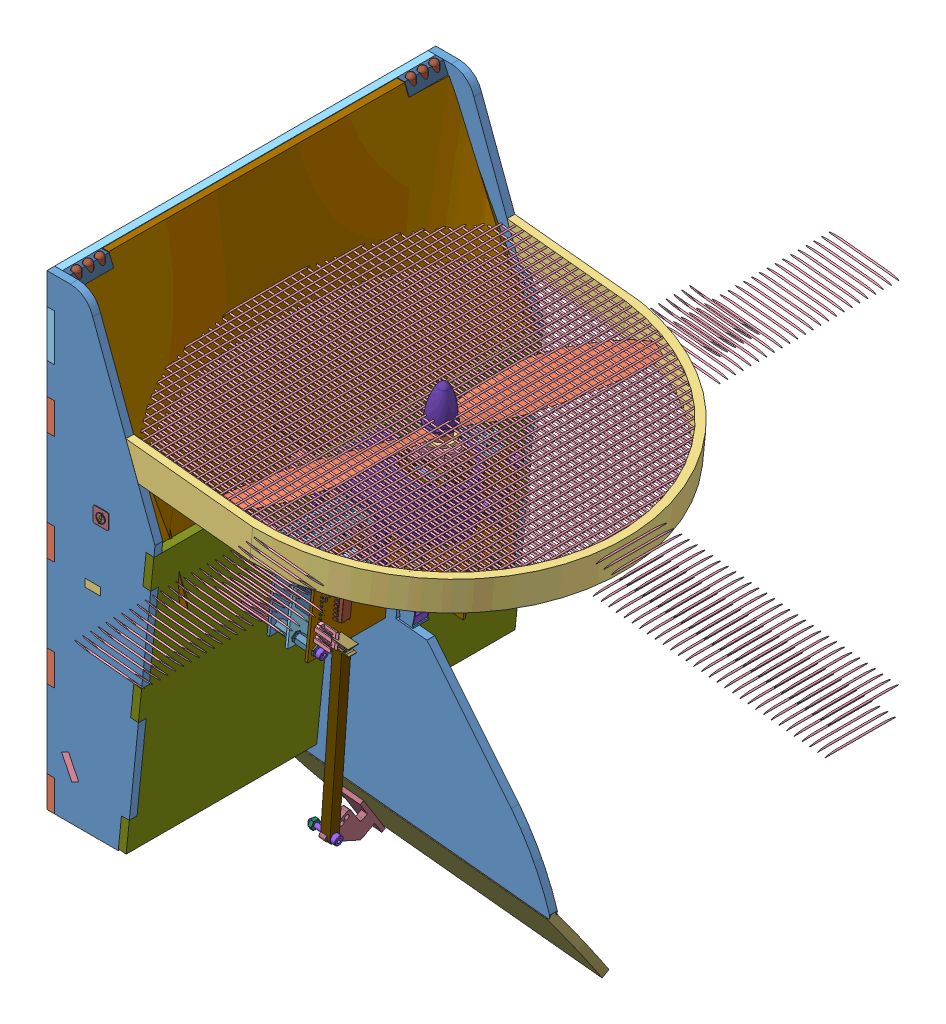
SolidWorks assembly AssTotaleSimu5, configuration Défaut. Lengths in mm.
Overall size (253.25 382.9 251.6).
1779 component instances, 238 part files, 11 mates.
Components (placement in the parent):
- AssStructSimu-1: AssStructSimu [Défaut] at (-125.7658 -1.8483 624.6548) x (1 0 0) z (0 0 -1) size (253.25 324.59 251.6)
  - AssBase-1: AssBase [Défaut] at (36.5482 -71.0398 34.0612) size (86.08 302.3 251.6)
    - AssD-1: AssD [Défaut] at (39.0992 31.0201 8.5) size (69.5 300 22)
      - P1-1: P1 [Défaut] at (-95.5819 194.6656 377.5) size (69.5 300 5)
      - P5-1: P5 [Défaut] at (-100.5819 -35.3344 360.5) x (0 1 0) z (1 0 0) size (230 22 5)
    - AssG-1: AssG [Défaut] at (39.0992 31.0201 -236.5) size (69.5 300 22)
      - P1-1: P1 [Défaut] at (-95.5819 194.6656 377.5) size (69.5 300 5)
      - P5-1: P5 [Défaut] at (-95.5819 -35.3344 399.5) x (0 1 0) z (-1 0 0) size (230 22 5)
    - P7-1: P7 [Défaut] at (-1.4828 89.6857 370.5) x (0 0 -1) z (0 -1 0) size (250 54.5 5)
    - P4-1: P4 [Défaut] at (-63.2363 165.9323 386) x (0 0 -1) z (0.898794 -0.438371 0) size (250 60.5 66.27)
    - P3-1: P3 [Défaut] at (-56.4828 -74.3143 146) x (0 0 1) z (-1 0 0) size (250 70 5)
    - P4b-1: P4b [Défaut] at (-58.7423 163.7404 190) x (0 0 1) z (0.438371 0.898794 0) size (152 56 2)
    - battery-1: battery [Défaut] at (-39.0156 204.1861 197.5) x (0 0 1) z (0.898794 -0.438371 0) size (137 43 30)
    - socket head cap screw 4762_din-1: socket head cap screw 4762_din [EN ISO 4762 M3 x 10 - 10N] at (-27.7008 145.2627 193) x (0.438371 0.898794 0) z (0 0 -1) size (13 5.5 5.5)
    - socket head cap screw 4762_din-2: socket head cap screw 4762_din [EN ISO 4762 M3 x 10 - 10N] at (-27.7008 145.2627 339) x (0.438371 0.898794 0) z (-0.791285 0.385936 -0.474259) size (13 5.5 5.5)
    - socket head cap screw 4762_din-3: socket head cap screw 4762_din [EN ISO 4762 M3 x 10 - 10N] at (-42.0815 152.2766 339) x (0.438371 0.898794 0) z (-0.001489 0.000726 -0.999999) size (13 5.5 5.5)
    - socket head cap screw 4762_din-4: socket head cap screw 4762_din [EN ISO 4762 M3 x 10 - 10N] at (-42.0815 152.2766 193) x (0.438371 0.898794 0) z (-0.031331 0.015281 -0.999392) size (13 5.5 5.5)
    - P11-1: P11 [Défaut] at (-57.5734 -73.9703 146.7843) x (0.005072 0 0.999987) z (0.006197 0.999981 -0.000031) size (240 65 164)
    - AssPhare-1: AssPhare [Défaut] at (-52.8518 -67.6977 411) x (0 1 0) z (0 0 -1) size (35.8 8 25)
      - piece_led-1: piece_led [Défaut] at (-6.6166 -3.631 25) size (7 8 25)
      - LED 5mm-1: LED 5mm [Valor predeterminado] at (-0.1166 0.369 30) x (0 0 1) z (-1 0 0) size (10.06 6 40.8)
      - LED 5mm-2: LED 5mm [Valor predeterminado] at (-0.1166 0.369 37.5) x (0 0 1) z (-1 0 0) size (10.06 6 40.8)
      - LED 5mm-3: LED 5mm [Valor predeterminado] at (-0.1166 0.369 45) x (0 0 1) z (-1 0 0) size (10.06 6 40.8)
    - AssPhare-2: AssPhare [Défaut] at (-52.8518 -67.6977 196) x (0 1 0) z (0 0 -1) size (35.8 8 25)
      - piece_led-1: piece_led [Défaut] at (-6.6166 -3.631 25) size (7 8 25)
      - LED 5mm-1: LED 5mm [Valor predeterminado] at (-0.1166 0.369 30) x (0 0 1) z (-1 0 0) size (10.06 6 40.8)
      - LED 5mm-2: LED 5mm [Valor predeterminado] at (-0.1166 0.369 37.5) x (0 0 1) z (-1 0 0) size (10.06 6 40.8)
      - LED 5mm-3: LED 5mm [Valor predeterminado] at (-0.1166 0.369 45) x (0 0 1) z (-1 0 0) size (10.06 6 40.8)
    - AssLogo-1: AssLogo [Défaut] at (-27.8835 45.1673 148.1054) x (-1 0 0) z (0 0 -1) size (10 10 0.8)
      - logo1-1: logo1 [Défaut] at (-6.5271 -4.4734 6.5054) size (5.8 7.71 0.4)
      - logo2-1: logo2 [Défaut] at (-6.4007 -4.4815 7.1054) size (10 10 0.4)
    - AssLogo-2: AssLogo [Défaut] at (-25.082 45.1673 383.8946) size (10 10 0.8)
      - logo1-1: logo1 [Défaut] at (-6.5271 -4.4734 6.5054) size (5.8 7.71 0.4)
      - logo2-1: logo2 [Défaut] at (-6.4007 -4.4815 7.1054) size (10 10 0.4)
    - support2-1: support2 [Défaut] at (-61.5648 191.7124 276) x (-0.017452 -0.999848 0) z (0.999848 -0.017452 0) size (75 20 10)
    - socket head cap screw 4762_din-5: socket head cap screw 4762_din [EN ISO 4762 M3 x 5 - 5N] at (-61.652 186.7132 269.3333) x (0.999848 -0.017452 0) z (-0.002158 -0.123615 0.992328) size (8 5.5 5.5)
    - socket head cap screw 4762_din-6: socket head cap screw 4762_din [EN ISO 4762 M3 x 5 - 5N] at (-61.652 186.7132 262.6667) x (0.999848 -0.017452 0) z (0 0 1) size (8 5.5 5.5)
    - socket head cap screw 4762_din-7: socket head cap screw 4762_din [EN ISO 4762 M3 x 25 - 18N] at (-55.2963 121.0922 253) x (0 0 1) z (-1 0 0) size (28 5.5 5.5)
    - hex nut style 1 gradeab_din-1: hex nut style 1 gradeab_din [Hexagon Nut ISO 4032 - M3 - W - N] at (-55.2963 121.0922 276) x (-0.923728 -0.383049 0) z (0 0 -1) size (5.5 6.35 2.4)
  - AssToitMot-1: AssToitMot [Défaut] at (-168.5238 43.6961 238.494) x (0 0 -1) z (0.9948 0.101852 0) size (250 207.5 205)
    - AssToit-1: AssToit [Défaut] at (-23.0702 -16.5789 -3.7148) size (250 207.5 205)
      - P8-1: P8 [Défaut] at (-38.4971 122.5921 203.5) size (250 175 5)
      - P12-1: P12 [Défaut] at (-60.4971 -63.4079 265.5) x (1 0 0) z (0 -1 0) size (44.28 76.64 55)
      - P13-1: P13 [Défaut] at (-35.9971 -52.8579 208.5) x (0 0 1) z (-1 0 0) size (64 15.55 5)
      - P10_2-1: P10_2 [Défaut] at (-35.9971 111.5921 171) x (0 0 1) z (-1 0 0) size (188.5 117.6 5)
    - Parallax-Servo_DUMMY-1: Parallax-Servo_DUMMY [Défaut] at (-61.6002 -51.5207 216.6662) x (1 0 0) z (0 1 0) size (20.07 42.67 55.64)
    - socket head cap screw 4762_din-1: socket head cap screw 4762_din [EN ISO 4762 M2.5 x 5 - 5N] at (-51.9272 -76.4868 259.2852) x (0 -1 0) z (-0.546944 0 0.837169) size (7.5 4.5 4.5)
    - socket head cap screw 4762_din-2: socket head cap screw 4762_din [EN ISO 4762 M2.5 x 5 - 5N] at (-61.5672 -76.4868 268.9252) x (0 -1 0) z (-0.546944 0 0.837169) size (7.5 4.5 4.5)
    - socket head cap screw 4762_din-3: socket head cap screw 4762_din [EN ISO 4762 M2.5 x 5 - 5N] at (-71.2072 -76.4868 259.2852) x (0 -1 0) z (-0.546944 0 0.837169) size (7.5 4.5 4.5)
    - socket head cap screw 4762_din-4: socket head cap screw 4762_din [EN ISO 4762 M2.5 x 5 - 5N] at (-61.5672 -76.4868 249.6452) x (0 -1 0) z (-0.546944 0 0.837169) size (7.5 4.5 4.5)
    - AssPhare-1: AssPhare [Défaut] at (8.4328 83.3966 196.1542) x (0 -1 0) z (1 0 0) size (35.8 8 25)
      - piece_led-1: piece_led [Défaut] at (-6.6166 -3.631 25) size (7 8 25)
      - LED 5mm-1: LED 5mm [Valor predeterminado] at (-0.1166 0.369 30) x (0 0 1) z (-1 0 0) size (10.06 6 40.8)
      - LED 5mm-2: LED 5mm [Valor predeterminado] at (-0.1166 0.369 37.5) x (0 0 1) z (-1 0 0) size (10.06 6 40.8)
      - LED 5mm-3: LED 5mm [Valor predeterminado] at (-0.1166 0.369 45) x (0 0 1) z (-1 0 0) size (10.06 6 40.8)
    - AssPhare-2: AssPhare [Défaut] at (-206.5672 83.3966 196.1542) x (0 -1 0) z (1 0 0) size (35.8 8 25)
      - piece_led-1: piece_led [Défaut] at (-6.6166 -3.631 25) size (7 8 25)
      - LED 5mm-1: LED 5mm [Valor predeterminado] at (-0.1166 0.369 30) x (0 0 1) z (-1 0 0) size (10.06 6 40.8)
      - LED 5mm-2: LED 5mm [Valor predeterminado] at (-0.1166 0.369 37.5) x (0 0 1) z (-1 0 0) size (10.06 6 40.8)
      - LED 5mm-3: LED 5mm [Valor predeterminado] at (-0.1166 0.369 45) x (0 0 1) z (-1 0 0) size (10.06 6 40.8)
    - socket head cap screw 4762_din-5: socket head cap screw 4762_din [EN ISO 4762 M3 x 10 - 10N] at (-67.0672 -22.9368 210.2852) x (0 0 -1) z (1 0 0) size (13 5.5 5.5)
    - socket head cap screw 4762_din-6: socket head cap screw 4762_din [EN ISO 4762 M3 x 10 - 10N] at (-56.0672 -72.9868 210.2852) x (0 0 -1) z (1 0 0) size (13 5.5 5.5)
    - socket head cap screw 4762_din-7: socket head cap screw 4762_din [EN ISO 4762 M3 x 10 - 10N] at (-67.0672 -72.9868 210.2852) x (0 0 -1) z (1 0 0) size (13 5.5 5.5)
    - socket head cap screw 4762_din-8: socket head cap screw 4762_din [EN ISO 4762 M3 x 10 - 10N] at (-56.0672 -22.9368 210.2852) x (0 0 -1) z (1 0 0) size (13 5.5 5.5)
    - hex nut style 1 gradeab_din-1: hex nut style 1 gradeab_din [Hexagon Nut ISO 4032 - M3 - W - N] at (-67.0672 -72.9868 197.3852) x (-0.923728 -0.383049 0) z (0 0 -1) size (5.5 6.35 2.4)
    - hex nut style 1 gradeab_din-2: hex nut style 1 gradeab_din [Hexagon Nut ISO 4032 - M3 - W - N] at (-56.0672 -72.9868 199.7852) size (5.5 6.35 2.4)
    - hex nut style 1 gradeab_din-3: hex nut style 1 gradeab_din [Hexagon Nut ISO 4032 - M3 - W - N] at (-67.0672 -22.9368 199.7852) size (5.5 6.35 2.4)
    - hex nut style 1 gradeab_din-4: hex nut style 1 gradeab_din [Hexagon Nut ISO 4032 - M3 - W - N] at (-56.0672 -22.9368 199.7852) size (5.5 6.35 2.4)
  - AssProtec-1: AssProtec [Défaut] at (86.6746 190.4649 284.6351) x (0 0 -1) z (0.101852 -0.9948 0) size (250 237.46 20)
    - protec3c-1: protec3c [Défaut] at (-140.4261 -87.7568 240) size (250 197 20)
    - AssGrillage-1: AssGrillage [Défaut] at (-370.4609 -132.5428 258.3161) x (0 0 -1) z (1 0 0) size (2.02 237.05 250)
      - barreau-1: barreau [Défaut] at (-1.1839 0.254 200) size (1 1 400)
      - barreau-3: barreau [Défaut] at (-1.1839 5.254 200) size (1 1 400)
      - barreau-4: barreau [Défaut] at (-1.1839 10.254 200) size (1 1 400)
      - barreau-5: barreau [Défaut] at (-1.1839 15.254 200) size (1 1 400)
      - barreau-6: barreau [Défaut] at (-1.1839 20.254 200) size (1 1 400)
      - barreau-7: barreau [Défaut] at (-1.1839 25.254 200) size (1 1 400)
      - barreau-8: barreau [Défaut] at (-1.1839 30.254 200) size (1 1 400)
      - barreau-9: barreau [Défaut] at (-1.1839 35.254 200) size (1 1 400)
      - barreau-10: barreau [Défaut] at (-1.1839 40.254 200) size (1 1 400)
      - barreau-11: barreau [Défaut] at (-1.1839 45.254 200) size (1 1 400)
      - barreau-12: barreau [Défaut] at (-1.1839 50.254 200) size (1 1 400)
      - barreau-13: barreau [Défaut] at (-1.1839 55.254 200) size (1 1 400)
      - barreau-14: barreau [Défaut] at (-1.1839 60.254 200) size (1 1 400)
      - barreau-15: barreau [Défaut] at (-1.1839 65.254 200) size (1 1 400)
      - barreau-16: barreau [Défaut] at (-1.1839 70.254 200) size (1 1 400)
      - barreau-17: barreau [Défaut] at (-1.1839 75.254 200) size (1 1 400)
      - barreau-18: barreau [Défaut] at (-1.1839 80.254 200) size (1 1 400)
      - barreau-19: barreau [Défaut] at (-1.1839 85.254 200) size (1 1 400)
      - barreau-20: barreau [Défaut] at (-1.1839 90.254 200) size (1 1 400)
      - barreau-21: barreau [Défaut] at (-1.1839 95.254 200) size (1 1 400)
      - barreau-22: barreau [Défaut] at (-1.1839 100.254 200) size (1 1 400)
      - barreau-23: barreau [Défaut] at (-1.1839 105.254 200) size (1 1 400)
      - barreau-24: barreau [Défaut] at (-1.1839 110.254 200) size (1 1 400)
      - barreau-25: barreau [Défaut] at (-1.1839 115.254 200) size (1 1 400)
      - barreau-26: barreau [Défaut] at (-1.1839 120.254 200) size (1 1 400)
      - barreau-27: barreau [Défaut] at (-1.1839 125.254 200) size (1 1 400)
      - barreau-28: barreau [Défaut] at (-1.1839 130.254 200) size (1 1 400)
      - barreau-29: barreau [Défaut] at (-1.1839 135.254 200) size (1 1 400)
      - barreau-30: barreau [Défaut] at (-1.1839 140.254 200) size (1 1 400)
      - barreau-31: barreau [Défaut] at (-1.1839 145.254 200) size (1 1 400)
      - barreau-32: barreau [Défaut] at (-1.1839 150.254 200) size (1 1 400)
      - barreau-33: barreau [Défaut] at (-1.1839 155.254 200) size (1 1 400)
      - barreau-34: barreau [Défaut] at (-1.1839 160.254 200) size (1 1 400)
      - barreau-35: barreau [Défaut] at (-1.1839 165.254 200) size (1 1 400)
      - barreau-36: barreau [Défaut] at (-1.1839 170.254 200) size (1 1 400)
      - barreau-37: barreau [Défaut] at (-1.1839 175.254 200) size (1 1 400)
      - barreau-38: barreau [Défaut] at (-1.1839 180.254 200) size (1 1 400)
      - barreau-39: barreau [Défaut] at (-1.1839 185.254 200) size (1 1 400)
      - barreau-40: barreau [Défaut] at (-1.1839 190.254 200) size (1 1 400)
      - barreau-41: barreau [Défaut] at (-1.1839 195.254 200) size (1 1 400)
      - barreau-42: barreau [Défaut] at (-0.1839 -1.5314 598.7823) x (0.998922 0 0.04641) z (0 1 0) size (1 1 400)
      - barreau-43: barreau [Défaut] at (-1.1839 200.254 200) size (1 1 400)
      - barreau-44: barreau [Défaut] at (-1.1839 205.254 200) size (1 1 400)
      - barreau-45: barreau [Défaut] at (-1.1839 210.254 200) size (1 1 400)
      - barreau-46: barreau [Défaut] at (-1.1839 215.254 200) size (1 1 400)
      - barreau-47: barreau [Défaut] at (-1.1839 220.254 200) size (1 1 400)
      - barreau-48: barreau [Défaut] at (-1.1839 225.254 200) size (1 1 400)
      - barreau-49: barreau [Défaut] at (-1.1839 230.254 200) size (1 1 400)
      - barreau-50: barreau [Défaut] at (-1.1839 235.254 200) size (1 1 400)
      - barreau-51: barreau [Défaut] at (-1.1839 240.254 200) size (1 1 400)
      - barreau-52: barreau [Défaut] at (-1.1839 245.254 200) size (1 1 400)
      - barreau-53: barreau [Défaut] at (-1.1839 250.254 200) size (1 1 400)
      - barreau-54: barreau [Défaut] at (-1.1839 255.254 200) size (1 1 400)
      - barreau-55: barreau [Défaut] at (-1.1839 260.254 200) size (1 1 400)
      - barreau-56: barreau [Défaut] at (-1.1839 265.254 200) size (1 1 400)
      - barreau-57: barreau [Défaut] at (-1.1839 270.254 200) size (1 1 400)
      - barreau-58: barreau [Défaut] at (-1.1839 275.254 200) size (1 1 400)
      - barreau-59: barreau [Défaut] at (-1.1839 280.254 200) size (1 1 400)
      - barreau-60: barreau [Défaut] at (-1.1839 285.254 200) size (1 1 400)
      - barreau-61: barreau [Défaut] at (-1.1839 290.254 200) size (1 1 400)
      - barreau-62: barreau [Défaut] at (-1.1839 295.254 200) size (1 1 400)
      - barreau-63: barreau [Défaut] at (-1.1839 300.254 200) size (1 1 400)
      - barreau-64: barreau [Défaut] at (-1.1839 305.254 200) size (1 1 400)
      - barreau-65: barreau [Défaut] at (-1.1839 310.254 200) size (1 1 400)
      - barreau-66: barreau [Défaut] at (-1.1839 315.254 200) size (1 1 400)
      - barreau-67: barreau [Défaut] at (-1.1839 320.254 200) size (1 1 400)
      - barreau-68: barreau [Défaut] at (-1.1839 325.254 200) size (1 1 400)
      - barreau-69: barreau [Défaut] at (-1.1839 330.254 200) size (1 1 400)
      - barreau-70: barreau [Défaut] at (-1.1839 335.254 200) size (1 1 400)
      - barreau-71: barreau [Défaut] at (-1.1839 340.254 200) size (1 1 400)
      - barreau-72: barreau [Défaut] at (-1.1839 345.254 200) size (1 1 400)
      - barreau-73: barreau [Défaut] at (-1.1839 350.254 200) size (1 1 400)
      - barreau-74: barreau [Défaut] at (-1.1839 355.254 200) size (1 1 400)
      - barreau-75: barreau [Défaut] at (-1.1839 360.254 200) size (1 1 400)
      - barreau-76: barreau [Défaut] at (-1.1839 365.254 200) size (1 1 400)
      - barreau-77: barreau [Défaut] at (-1.1839 370.254 200) size (1 1 400)
      - barreau-78: barreau [Défaut] at (-1.1839 375.254 200) size (1 1 400)
      - barreau-79: barreau [Défaut] at (-1.1839 380.254 200) size (1 1 400)
      - barreau-80: barreau [Défaut] at (-1.1839 385.254 200) size (1 1 400)
      - barreau-81: barreau [Défaut] at (-1.1839 390.254 200) size (1 1 400)
      - barreau-82: barreau [Défaut] at (-1.1839 395.254 200) size (1 1 400)
      - barreau-136: barreau [Défaut] at (-0.1839 -1.5314 593.7823) x (0.998922 0 0.04641) z (0 1 0) size (1 1 400)
      - barreau-137: barreau [Défaut] at (-0.1839 -1.5314 588.7823) x (0.998922 0 0.04641) z (0 1 0) size (1 1 400)
      - barreau-138: barreau [Défaut] at (-0.1839 -1.5314 583.7823) x (0.998922 0 0.04641) z (0 1 0) size (1 1 400)
      - barreau-139: barreau [Défaut] at (-0.1839 -1.5314 578.7823) x (0.998922 0 0.04641) z (0 1 0) size (1 1 400)
      - barreau-140: barreau [Défaut] at (-0.1839 -1.5314 573.7823) x (0.998922 0 0.04641) z (0 1 0) size (1 1 400)
      - barreau-141: barreau [Défaut] at (-0.1839 -1.5314 568.7823) x (0.998922 0 0.04641) z (0 1 0) size (1 1 400)
      - barreau-142: barreau [Défaut] at (-0.1839 -1.5314 563.7823) x (0.998922 0 0.04641) z (0 1 0) size (1 1 400)
      - barreau-143: barreau [Défaut] at (-0.1839 -1.5314 558.7823) x (0.998922 0 0.04641) z (0 1 0) size (1 1 400)
      - barreau-144: barreau [Défaut] at (-0.1839 -1.5314 553.7823) x (0.998922 0 0.04641) z (0 1 0) size (1 1 400)
      - barreau-145: barreau [Défaut] at (-0.1839 -1.5314 548.7823) x (0.998922 0 0.04641) z (0 1 0) size (1 1 400)
      - barreau-146: barreau [Défaut] at (-0.1839 -1.5314 543.7823) x (0.998922 0 0.04641) z (0 1 0) size (1 1 400)
      - barreau-147: barreau [Défaut] at (-0.1839 -1.5314 538.7823) x (0.998922 0 0.04641) z (0 1 0) size (1 1 400)
      - barreau-148: barreau [Défaut] at (-0.1839 -1.5314 533.7823) x (0.998922 0 0.04641) z (0 1 0) size (1 1 400)
      - barreau-149: barreau [Défaut] at (-0.1839 -1.5314 528.7823) x (0.998922 0 0.04641) z (0 1 0) size (1 1 400)
      - barreau-150: barreau [Défaut] at (-0.1839 -1.5314 523.7823) x (0.998922 0 0.04641) z (0 1 0) size (1 1 400)
      - barreau-151: barreau [Défaut] at (-0.1839 -1.5314 518.7823) x (0.998922 0 0.04641) z (0 1 0) size (1 1 400)
      - barreau-152: barreau [Défaut] at (-0.1839 -1.5314 513.7823) x (0.998922 0 0.04641) z (0 1 0) size (1 1 400)
      - barreau-153: barreau [Défaut] at (-0.1839 -1.5314 508.7823) x (0.998922 0 0.04641) z (0 1 0) size (1 1 400)
      - barreau-154: barreau [Défaut] at (-0.1839 -1.5314 503.7823) x (0.998922 0 0.04641) z (0 1 0) size (1 1 400)
      - barreau-155: barreau [Défaut] at (-0.1839 -1.5314 498.7823) x (0.998922 0 0.04641) z (0 1 0) size (1 1 400)
      - barreau-156: barreau [Défaut] at (-0.1839 -1.5314 493.7823) x (0.998922 0 0.04641) z (0 1 0) size (1 1 400)
      - barreau-157: barreau [Défaut] at (-0.1839 -1.5314 488.7823) x (0.998922 0 0.04641) z (0 1 0) size (1 1 400)
      - barreau-158: barreau [Défaut] at (-0.1839 -1.5314 483.7823) x (0.998922 0 0.04641) z (0 1 0) size (1 1 400)
      - barreau-159: barreau [Défaut] at (-0.1839 -1.5314 478.7823) x (0.998922 0 0.04641) z (0 1 0) size (1 1 400)
      - barreau-160: barreau [Défaut] at (-0.1839 -1.5314 473.7823) x (0.998922 0 0.04641) z (0 1 0) size (1 1 400)
      - barreau-161: barreau [Défaut] at (-0.1839 -1.5314 468.7823) x (0.998922 0 0.04641) z (0 1 0) size (1 1 400)
      - barreau-162: barreau [Défaut] at (-0.1839 -1.5314 463.7823) x (0.998922 0 0.04641) z (0 1 0) size (1 1 400)
      - barreau-163: barreau [Défaut] at (-0.1839 -1.5314 458.7823) x (0.998922 0 0.04641) z (0 1 0) size (1 1 400)
      - barreau-164: barreau [Défaut] at (-0.1839 -1.5314 453.7823) x (0.998922 0 0.04641) z (0 1 0) size (1 1 400)
      - barreau-165: barreau [Défaut] at (-0.1839 -1.5314 448.7823) x (0.998922 0 0.04641) z (0 1 0) size (1 1 400)
      - barreau-166: barreau [Défaut] at (-0.1839 -1.5314 443.7823) x (0.998922 0 0.04641) z (0 1 0) size (1 1 400)
      - barreau-167: barreau [Défaut] at (-0.1839 -1.5314 438.7823) x (0.998922 0 0.04641) z (0 1 0) size (1 1 400)
      - barreau-168: barreau [Défaut] at (-0.1839 -1.5314 433.7823) x (0.998922 0 0.04641) z (0 1 0) size (1 1 400)
      - barreau-169: barreau [Défaut] at (-0.1839 -1.5314 428.7823) x (0.998922 0 0.04641) z (0 1 0) size (1 1 400)
      - barreau-170: barreau [Défaut] at (-0.1839 -1.5314 423.7823) x (0.998922 0 0.04641) z (0 1 0) size (1 1 400)
      - barreau-171: barreau [Défaut] at (-0.1839 -1.5314 418.7823) x (0.998922 0 0.04641) z (0 1 0) size (1 1 400)
      - barreau-172: barreau [Défaut] at (-0.1839 -1.5314 413.7823) x (0.998922 0 0.04641) z (0 1 0) size (1 1 400)
      - barreau-173: barreau [Défaut] at (-0.1839 -1.5314 408.7823) x (0.998922 0 0.04641) z (0 1 0) size (1 1 400)
      - barreau-174: barreau [Défaut] at (-0.1839 -1.5314 403.7823) x (0.998922 0 0.04641) z (0 1 0) size (1 1 400)
      - barreau-175: barreau [Défaut] at (-0.1839 -1.5314 398.7823) x (0.998922 0 0.04641) z (0 1 0) size (1 1 400)
      - barreau-176: barreau [Défaut] at (-0.1839 -1.5314 393.7823) x (0.998922 0 0.04641) z (0 1 0) size (1 1 400)
      - barreau-177: barreau [Défaut] at (-0.1839 -1.5314 388.7823) x (0.998922 0 0.04641) z (0 1 0) size (1 1 400)
      - barreau-178: barreau [Défaut] at (-0.1839 -1.5314 383.7823) x (0.998922 0 0.04641) z (0 1 0) size (1 1 400)
      - barreau-179: barreau [Défaut] at (-0.1839 -1.5314 378.7823) x (0.998922 0 0.04641) z (0 1 0) size (1 1 400)
      - barreau-180: barreau [Défaut] at (-0.1839 -1.5314 373.7823) x (0.998922 0 0.04641) z (0 1 0) size (1 1 400)
      - barreau-181: barreau [Défaut] at (-0.1839 -1.5314 368.7823) x (0.998922 0 0.04641) z (0 1 0) size (1 1 400)
      - barreau-182: barreau [Défaut] at (-0.1839 -1.5314 363.7823) x (0.998922 0 0.04641) z (0 1 0) size (1 1 400)
      - barreau-183: barreau [Défaut] at (-0.1839 -1.5314 358.7823) x (0.998922 0 0.04641) z (0 1 0) size (1 1 400)
      - barreau-184: barreau [Défaut] at (-0.1839 -1.5314 353.7823) x (0.998922 0 0.04641) z (0 1 0) size (1 1 400)
      - barreau-185: barreau [Défaut] at (-0.1839 -1.5314 348.7823) x (0.998922 0 0.04641) z (0 1 0) size (1 1 400)
      - barreau-186: barreau [Défaut] at (-0.1839 -1.5314 343.7823) x (0.998922 0 0.04641) z (0 1 0) size (1 1 400)
      - barreau-187: barreau [Défaut] at (-0.1839 -1.5314 338.7823) x (0.998922 0 0.04641) z (0 1 0) size (1 1 400)
      - barreau-188: barreau [Défaut] at (-0.1839 -1.5314 333.7823) x (0.998922 0 0.04641) z (0 1 0) size (1 1 400)
      - barreau-189: barreau [Défaut] at (-0.1839 -1.5314 328.7823) x (0.998922 0 0.04641) z (0 1 0) size (1 1 400)
      - barreau-190: barreau [Défaut] at (-0.1839 -1.5314 323.7823) x (0.998922 0 0.04641) z (0 1 0) size (1 1 400)
      - barreau-191: barreau [Défaut] at (-0.1839 -1.5314 318.7823) x (0.998922 0 0.04641) z (0 1 0) size (1 1 400)
      - barreau-192: barreau [Défaut] at (-0.1839 -1.5314 313.7823) x (0.998922 0 0.04641) z (0 1 0) size (1 1 400)
      - barreau-193: barreau [Défaut] at (-0.1839 -1.5314 308.7823) x (0.998922 0 0.04641) z (0 1 0) size (1 1 400)
      - barreau-194: barreau [Défaut] at (-0.1839 -1.5314 303.7823) x (0.998922 0 0.04641) z (0 1 0) size (1 1 400)
      - barreau-195: barreau [Défaut] at (-0.1839 -1.5314 298.7823) x (0.998922 0 0.04641) z (0 1 0) size (1 1 400)
      - barreau-196: barreau [Défaut] at (-0.1839 -1.5314 293.7823) x (0.998922 0 0.04641) z (0 1 0) size (1 1 400)
      - barreau-197: barreau [Défaut] at (-0.1839 -1.5314 288.7823) x (0.998922 0 0.04641) z (0 1 0) size (1 1 400)
      - barreau-198: barreau [Défaut] at (-0.1839 -1.5314 283.7823) x (0.998922 0 0.04641) z (0 1 0) size (1 1 400)
      - barreau-199: barreau [Défaut] at (-0.1839 -1.5314 278.7823) x (0.998922 0 0.04641) z (0 1 0) size (1 1 400)
      - barreau-200: barreau [Défaut] at (-0.1839 -1.5314 273.7823) x (0.998922 0 0.04641) z (0 1 0) size (1 1 400)
      - barreau-201: barreau [Défaut] at (-0.1839 -1.5314 268.7823) x (0.998922 0 0.04641) z (0 1 0) size (1 1 400)
      - barreau-202: barreau [Défaut] at (-0.1839 -1.5314 263.7823) x (0.998922 0 0.04641) z (0 1 0) size (1 1 400)
      - barreau-203: barreau [Défaut] at (-0.1839 -1.5314 258.7823) x (0.998922 0 0.04641) z (0 1 0) size (1 1 400)
      - barreau-204: barreau [Défaut] at (-0.1839 -1.5314 253.7823) x (0.998922 0 0.04641) z (0 1 0) size (1 1 400)
      - barreau-205: barreau [Défaut] at (-0.1839 -1.5314 248.7823) x (0.998922 0 0.04641) z (0 1 0) size (1 1 400)
      - barreau-206: barreau [Défaut] at (-0.1839 -1.5314 243.7823) x (0.998922 0 0.04641) z (0 1 0) size (1 1 400)
      - barreau-207: barreau [Défaut] at (-0.1839 -1.5314 238.7823) x (0.998922 0 0.04641) z (0 1 0) size (1 1 400)
      - barreau-208: barreau [Défaut] at (-0.1839 -1.5314 233.7823) x (0.998922 0 0.04641) z (0 1 0) size (1 1 400)
      - barreau-209: barreau [Défaut] at (-0.1839 -1.5314 228.7823) x (0.998922 0 0.04641) z (0 1 0) size (1 1 400)
      - barreau-210: barreau [Défaut] at (-0.1839 -1.5314 223.7823) x (0.998922 0 0.04641) z (0 1 0) size (1 1 400)
      - barreau-211: barreau [Défaut] at (-0.1839 -1.5314 218.7823) x (0.998922 0 0.04641) z (0 1 0) size (1 1 400)
      - barreau-212: barreau [Défaut] at (-0.1839 -1.5314 213.7823) x (0.998922 0 0.04641) z (0 1 0) size (1 1 400)
      - barreau-213: barreau [Défaut] at (-0.1839 -1.5314 208.7823) x (0.998922 0 0.04641) z (0 1 0) size (1 1 400)
      - barreau-214: barreau [Défaut] at (-0.1839 -1.5314 203.7823) x (0.998922 0 0.04641) z (0 1 0) size (1 1 400)
    - AssGrillage-2: AssGrillage [Défaut] at (339.6086 -132.5428 241.6839) x (0 0 1) z (-1 0 0) size (2.02 237.05 250)
      - barreau-1: barreau [Défaut] at (-1.1839 0.254 200) size (1 1 400)
      - barreau-3: barreau [Défaut] at (-1.1839 5.254 200) size (1 1 400)
      - barreau-4: barreau [Défaut] at (-1.1839 10.254 200) size (1 1 400)
      - barreau-5: barreau [Défaut] at (-1.1839 15.254 200) size (1 1 400)
      - barreau-6: barreau [Défaut] at (-1.1839 20.254 200) size (1 1 400)
      - barreau-7: barreau [Défaut] at (-1.1839 25.254 200) size (1 1 400)
      - barreau-8: barreau [Défaut] at (-1.1839 30.254 200) size (1 1 400)
      - barreau-9: barreau [Défaut] at (-1.1839 35.254 200) size (1 1 400)
      - barreau-10: barreau [Défaut] at (-1.1839 40.254 200) size (1 1 400)
      - barreau-11: barreau [Défaut] at (-1.1839 45.254 200) size (1 1 400)
      - barreau-12: barreau [Défaut] at (-1.1839 50.254 200) size (1 1 400)
      - barreau-13: barreau [Défaut] at (-1.1839 55.254 200) size (1 1 400)
      - barreau-14: barreau [Défaut] at (-1.1839 60.254 200) size (1 1 400)
      - barreau-15: barreau [Défaut] at (-1.1839 65.254 200) size (1 1 400)
      - barreau-16: barreau [Défaut] at (-1.1839 70.254 200) size (1 1 400)
      - barreau-17: barreau [Défaut] at (-1.1839 75.254 200) size (1 1 400)
      - barreau-18: barreau [Défaut] at (-1.1839 80.254 200) size (1 1 400)
      - barreau-19: barreau [Défaut] at (-1.1839 85.254 200) size (1 1 400)
      - barreau-20: barreau [Défaut] at (-1.1839 90.254 200) size (1 1 400)
      - barreau-21: barreau [Défaut] at (-1.1839 95.254 200) size (1 1 400)
      - barreau-22: barreau [Défaut] at (-1.1839 100.254 200) size (1 1 400)
      - barreau-23: barreau [Défaut] at (-1.1839 105.254 200) size (1 1 400)
      - barreau-24: barreau [Défaut] at (-1.1839 110.254 200) size (1 1 400)
      - barreau-25: barreau [Défaut] at (-1.1839 115.254 200) size (1 1 400)
      - barreau-26: barreau [Défaut] at (-1.1839 120.254 200) size (1 1 400)
      - barreau-27: barreau [Défaut] at (-1.1839 125.254 200) size (1 1 400)
      - barreau-28: barreau [Défaut] at (-1.1839 130.254 200) size (1 1 400)
      - barreau-29: barreau [Défaut] at (-1.1839 135.254 200) size (1 1 400)
      - barreau-30: barreau [Défaut] at (-1.1839 140.254 200) size (1 1 400)
      - barreau-31: barreau [Défaut] at (-1.1839 145.254 200) size (1 1 400)
      - barreau-32: barreau [Défaut] at (-1.1839 150.254 200) size (1 1 400)
      - barreau-33: barreau [Défaut] at (-1.1839 155.254 200) size (1 1 400)
      - barreau-34: barreau [Défaut] at (-1.1839 160.254 200) size (1 1 400)
      - barreau-35: barreau [Défaut] at (-1.1839 165.254 200) size (1 1 400)
      - barreau-36: barreau [Défaut] at (-1.1839 170.254 200) size (1 1 400)
      - barreau-37: barreau [Défaut] at (-1.1839 175.254 200) size (1 1 400)
      - barreau-38: barreau [Défaut] at (-1.1839 180.254 200) size (1 1 400)
      - barreau-39: barreau [Défaut] at (-1.1839 185.254 200) size (1 1 400)
      - barreau-40: barreau [Défaut] at (-1.1839 190.254 200) size (1 1 400)
      - barreau-41: barreau [Défaut] at (-1.1839 195.254 200) size (1 1 400)
      - barreau-42: barreau [Défaut] at (-0.1839 -1.5314 598.7823) x (0.998922 0 0.04641) z (0 1 0) size (1 1 400)
      - barreau-43: barreau [Défaut] at (-1.1839 200.254 200) size (1 1 400)
      - barreau-44: barreau [Défaut] at (-1.1839 205.254 200) size (1 1 400)
      - barreau-45: barreau [Défaut] at (-1.1839 210.254 200) size (1 1 400)
      - barreau-46: barreau [Défaut] at (-1.1839 215.254 200) size (1 1 400)
      - barreau-47: barreau [Défaut] at (-1.1839 220.254 200) size (1 1 400)
      - barreau-48: barreau [Défaut] at (-1.1839 225.254 200) size (1 1 400)
      - barreau-49: barreau [Défaut] at (-1.1839 230.254 200) size (1 1 400)
      - barreau-50: barreau [Défaut] at (-1.1839 235.254 200) size (1 1 400)
      - barreau-51: barreau [Défaut] at (-1.1839 240.254 200) size (1 1 400)
      - barreau-52: barreau [Défaut] at (-1.1839 245.254 200) size (1 1 400)
      - barreau-53: barreau [Défaut] at (-1.1839 250.254 200) size (1 1 400)
      - barreau-54: barreau [Défaut] at (-1.1839 255.254 200) size (1 1 400)
      - barreau-55: barreau [Défaut] at (-1.1839 260.254 200) size (1 1 400)
      - barreau-56: barreau [Défaut] at (-1.1839 265.254 200) size (1 1 400)
      - barreau-57: barreau [Défaut] at (-1.1839 270.254 200) size (1 1 400)
      - barreau-58: barreau [Défaut] at (-1.1839 275.254 200) size (1 1 400)
      - barreau-59: barreau [Défaut] at (-1.1839 280.254 200) size (1 1 400)
      - barreau-60: barreau [Défaut] at (-1.1839 285.254 200) size (1 1 400)
      - barreau-61: barreau [Défaut] at (-1.1839 290.254 200) size (1 1 400)
      - barreau-62: barreau [Défaut] at (-1.1839 295.254 200) size (1 1 400)
      - barreau-63: barreau [Défaut] at (-1.1839 300.254 200) size (1 1 400)
      - barreau-64: barreau [Défaut] at (-1.1839 305.254 200) size (1 1 400)
      - barreau-65: barreau [Défaut] at (-1.1839 310.254 200) size (1 1 400)
      - barreau-66: barreau [Défaut] at (-1.1839 315.254 200) size (1 1 400)
      - barreau-67: barreau [Défaut] at (-1.1839 320.254 200) size (1 1 400)
      - barreau-68: barreau [Défaut] at (-1.1839 325.254 200) size (1 1 400)
      - barreau-69: barreau [Défaut] at (-1.1839 330.254 200) size (1 1 400)
      - barreau-70: barreau [Défaut] at (-1.1839 335.254 200) size (1 1 400)
      - barreau-71: barreau [Défaut] at (-1.1839 340.254 200) size (1 1 400)
      - barreau-72: barreau [Défaut] at (-1.1839 345.254 200) size (1 1 400)
      - barreau-73: barreau [Défaut] at (-1.1839 350.254 200) size (1 1 400)
      - barreau-74: barreau [Défaut] at (-1.1839 355.254 200) size (1 1 400)
      - barreau-75: barreau [Défaut] at (-1.1839 360.254 200) size (1 1 400)
      - barreau-76: barreau [Défaut] at (-1.1839 365.254 200) size (1 1 400)
      - barreau-77: barreau [Défaut] at (-1.1839 370.254 200) size (1 1 400)
      - barreau-78: barreau [Défaut] at (-1.1839 375.254 200) size (1 1 400)
      - barreau-79: barreau [Défaut] at (-1.1839 380.254 200) size (1 1 400)
      - barreau-80: barreau [Défaut] at (-1.1839 385.254 200) size (1 1 400)
      - barreau-81: barreau [Défaut] at (-1.1839 390.254 200) size (1 1 400)
      - barreau-82: barreau [Défaut] at (-1.1839 395.254 200) size (1 1 400)
      - barreau-136: barreau [Défaut] at (-0.1839 -1.5314 593.7823) x (0.998922 0 0.04641) z (0 1 0) size (1 1 400)
      - barreau-137: barreau [Défaut] at (-0.1839 -1.5314 588.7823) x (0.998922 0 0.04641) z (0 1 0) size (1 1 400)
      - barreau-138: barreau [Défaut] at (-0.1839 -1.5314 583.7823) x (0.998922 0 0.04641) z (0 1 0) size (1 1 400)
      - barreau-139: barreau [Défaut] at (-0.1839 -1.5314 578.7823) x (0.998922 0 0.04641) z (0 1 0) size (1 1 400)
      - barreau-140: barreau [Défaut] at (-0.1839 -1.5314 573.7823) x (0.998922 0 0.04641) z (0 1 0) size (1 1 400)
      - barreau-141: barreau [Défaut] at (-0.1839 -1.5314 568.7823) x (0.998922 0 0.04641) z (0 1 0) size (1 1 400)
      - barreau-142: barreau [Défaut] at (-0.1839 -1.5314 563.7823) x (0.998922 0 0.04641) z (0 1 0) size (1 1 400)
      - barreau-143: barreau [Défaut] at (-0.1839 -1.5314 558.7823) x (0.998922 0 0.04641) z (0 1 0) size (1 1 400)
      - barreau-144: barreau [Défaut] at (-0.1839 -1.5314 553.7823) x (0.998922 0 0.04641) z (0 1 0) size (1 1 400)
      - barreau-145: barreau [Défaut] at (-0.1839 -1.5314 548.7823) x (0.998922 0 0.04641) z (0 1 0) size (1 1 400)
      - barreau-146: barreau [Défaut] at (-0.1839 -1.5314 543.7823) x (0.998922 0 0.04641) z (0 1 0) size (1 1 400)
      - barreau-147: barreau [Défaut] at (-0.1839 -1.5314 538.7823) x (0.998922 0 0.04641) z (0 1 0) size (1 1 400)
      - barreau-148: barreau [Défaut] at (-0.1839 -1.5314 533.7823) x (0.998922 0 0.04641) z (0 1 0) size (1 1 400)
      - barreau-149: barreau [Défaut] at (-0.1839 -1.5314 528.7823) x (0.998922 0 0.04641) z (0 1 0) size (1 1 400)
      - barreau-150: barreau [Défaut] at (-0.1839 -1.5314 523.7823) x (0.998922 0 0.04641) z (0 1 0) size (1 1 400)
      - barreau-151: barreau [Défaut] at (-0.1839 -1.5314 518.7823) x (0.998922 0 0.04641) z (0 1 0) size (1 1 400)
      - barreau-152: barreau [Défaut] at (-0.1839 -1.5314 513.7823) x (0.998922 0 0.04641) z (0 1 0) size (1 1 400)
      - barreau-153: barreau [Défaut] at (-0.1839 -1.5314 508.7823) x (0.998922 0 0.04641) z (0 1 0) size (1 1 400)
      - barreau-154: barreau [Défaut] at (-0.1839 -1.5314 503.7823) x (0.998922 0 0.04641) z (0 1 0) size (1 1 400)
      - barreau-155: barreau [Défaut] at (-0.1839 -1.5314 498.7823) x (0.998922 0 0.04641) z (0 1 0) size (1 1 400)
      - barreau-156: barreau [Défaut] at (-0.1839 -1.5314 493.7823) x (0.998922 0 0.04641) z (0 1 0) size (1 1 400)
      - barreau-157: barreau [Défaut] at (-0.1839 -1.5314 488.7823) x (0.998922 0 0.04641) z (0 1 0) size (1 1 400)
      - barreau-158: barreau [Défaut] at (-0.1839 -1.5314 483.7823) x (0.998922 0 0.04641) z (0 1 0) size (1 1 400)
      - barreau-159: barreau [Défaut] at (-0.1839 -1.5314 478.7823) x (0.998922 0 0.04641) z (0 1 0) size (1 1 400)
      - barreau-160: barreau [Défaut] at (-0.1839 -1.5314 473.7823) x (0.998922 0 0.04641) z (0 1 0) size (1 1 400)
      - barreau-161: barreau [Défaut] at (-0.1839 -1.5314 468.7823) x (0.998922 0 0.04641) z (0 1 0) size (1 1 400)
      - barreau-162: barreau [Défaut] at (-0.1839 -1.5314 463.7823) x (0.998922 0 0.04641) z (0 1 0) size (1 1 400)
      - barreau-163: barreau [Défaut] at (-0.1839 -1.5314 458.7823) x (0.998922 0 0.04641) z (0 1 0) size (1 1 400)
      - barreau-164: barreau [Défaut] at (-0.1839 -1.5314 453.7823) x (0.998922 0 0.04641) z (0 1 0) size (1 1 400)
      - barreau-165: barreau [Défaut] at (-0.1839 -1.5314 448.7823) x (0.998922 0 0.04641) z (0 1 0) size (1 1 400)
      - barreau-166: barreau [Défaut] at (-0.1839 -1.5314 443.7823) x (0.998922 0 0.04641) z (0 1 0) size (1 1 400)
      - barreau-167: barreau [Défaut] at (-0.1839 -1.5314 438.7823) x (0.998922 0 0.04641) z (0 1 0) size (1 1 400)
      - barreau-168: barreau [Défaut] at (-0.1839 -1.5314 433.7823) x (0.998922 0 0.04641) z (0 1 0) size (1 1 400)
      - barreau-169: barreau [Défaut] at (-0.1839 -1.5314 428.7823) x (0.998922 0 0.04641) z (0 1 0) size (1 1 400)
      - barreau-170: barreau [Défaut] at (-0.1839 -1.5314 423.7823) x (0.998922 0 0.04641) z (0 1 0) size (1 1 400)
      - barreau-171: barreau [Défaut] at (-0.1839 -1.5314 418.7823) x (0.998922 0 0.04641) z (0 1 0) size (1 1 400)
      - barreau-172: barreau [Défaut] at (-0.1839 -1.5314 413.7823) x (0.998922 0 0.04641) z (0 1 0) size (1 1 400)
      - barreau-173: barreau [Défaut] at (-0.1839 -1.5314 408.7823) x (0.998922 0 0.04641) z (0 1 0) size (1 1 400)
      - barreau-174: barreau [Défaut] at (-0.1839 -1.5314 403.7823) x (0.998922 0 0.04641) z (0 1 0) size (1 1 400)
      - barreau-175: barreau [Défaut] at (-0.1839 -1.5314 398.7823) x (0.998922 0 0.04641) z (0 1 0) size (1 1 400)
      - barreau-176: barreau [Défaut] at (-0.1839 -1.5314 393.7823) x (0.998922 0 0.04641) z (0 1 0) size (1 1 400)
      - barreau-177: barreau [Défaut] at (-0.1839 -1.5314 388.7823) x (0.998922 0 0.04641) z (0 1 0) size (1 1 400)
      - barreau-178: barreau [Défaut] at (-0.1839 -1.5314 383.7823) x (0.998922 0 0.04641) z (0 1 0) size (1 1 400)
      - barreau-179: barreau [Défaut] at (-0.1839 -1.5314 378.7823) x (0.998922 0 0.04641) z (0 1 0) size (1 1 400)
      - barreau-180: barreau [Défaut] at (-0.1839 -1.5314 373.7823) x (0.998922 0 0.04641) z (0 1 0) size (1 1 400)
      - barreau-181: barreau [Défaut] at (-0.1839 -1.5314 368.7823) x (0.998922 0 0.04641) z (0 1 0) size (1 1 400)
      - barreau-182: barreau [Défaut] at (-0.1839 -1.5314 363.7823) x (0.998922 0 0.04641) z (0 1 0) size (1 1 400)
      - barreau-183: barreau [Défaut] at (-0.1839 -1.5314 358.7823) x (0.998922 0 0.04641) z (0 1 0) size (1 1 400)
      - barreau-184: barreau [Défaut] at (-0.1839 -1.5314 353.7823) x (0.998922 0 0.04641) z (0 1 0) size (1 1 400)
      - barreau-185: barreau [Défaut] at (-0.1839 -1.5314 348.7823) x (0.998922 0 0.04641) z (0 1 0) size (1 1 400)
      - barreau-186: barreau [Défaut] at (-0.1839 -1.5314 343.7823) x (0.998922 0 0.04641) z (0 1 0) size (1 1 400)
      - barreau-187: barreau [Défaut] at (-0.1839 -1.5314 338.7823) x (0.998922 0 0.04641) z (0 1 0) size (1 1 400)
      - barreau-188: barreau [Défaut] at (-0.1839 -1.5314 333.7823) x (0.998922 0 0.04641) z (0 1 0) size (1 1 400)
      - barreau-189: barreau [Défaut] at (-0.1839 -1.5314 328.7823) x (0.998922 0 0.04641) z (0 1 0) size (1 1 400)
      - barreau-190: barreau [Défaut] at (-0.1839 -1.5314 323.7823) x (0.998922 0 0.04641) z (0 1 0) size (1 1 400)
      - barreau-191: barreau [Défaut] at (-0.1839 -1.5314 318.7823) x (0.998922 0 0.04641) z (0 1 0) size (1 1 400)
      - barreau-192: barreau [Défaut] at (-0.1839 -1.5314 313.7823) x (0.998922 0 0.04641) z (0 1 0) size (1 1 400)
      - barreau-193: barreau [Défaut] at (-0.1839 -1.5314 308.7823) x (0.998922 0 0.04641) z (0 1 0) size (1 1 400)
      - barreau-194: barreau [Défaut] at (-0.1839 -1.5314 303.7823) x (0.998922 0 0.04641) z (0 1 0) size (1 1 400)
      - barreau-195: barreau [Défaut] at (-0.1839 -1.5314 298.7823) x (0.998922 0 0.04641) z (0 1 0) size (1 1 400)
      - barreau-196: barreau [Défaut] at (-0.1839 -1.5314 293.7823) x (0.998922 0 0.04641) z (0 1 0) size (1 1 400)
      - barreau-197: barreau [Défaut] at (-0.1839 -1.5314 288.7823) x (0.998922 0 0.04641) z (0 1 0) size (1 1 400)
      - barreau-198: barreau [Défaut] at (-0.1839 -1.5314 283.7823) x (0.998922 0 0.04641) z (0 1 0) size (1 1 400)
      - barreau-199: barreau [Défaut] at (-0.1839 -1.5314 278.7823) x (0.998922 0 0.04641) z (0 1 0) size (1 1 400)
      - barreau-200: barreau [Défaut] at (-0.1839 -1.5314 273.7823) x (0.998922 0 0.04641) z (0 1 0) size (1 1 400)
      - barreau-201: barreau [Défaut] at (-0.1839 -1.5314 268.7823) x (0.998922 0 0.04641) z (0 1 0) size (1 1 400)
      - barreau-202: barreau [Défaut] at (-0.1839 -1.5314 263.7823) x (0.998922 0 0.04641) z (0 1 0) size (1 1 400)
      - barreau-203: barreau [Défaut] at (-0.1839 -1.5314 258.7823) x (0.998922 0 0.04641) z (0 1 0) size (1 1 400)
      - barreau-204: barreau [Défaut] at (-0.1839 -1.5314 253.7823) x (0.998922 0 0.04641) z (0 1 0) size (1 1 400)
      - barreau-205: barreau [Défaut] at (-0.1839 -1.5314 248.7823) x (0.998922 0 0.04641) z (0 1 0) size (1 1 400)
      - barreau-206: barreau [Défaut] at (-0.1839 -1.5314 243.7823) x (0.998922 0 0.04641) z (0 1 0) size (1 1 400)
      - barreau-207: barreau [Défaut] at (-0.1839 -1.5314 238.7823) x (0.998922 0 0.04641) z (0 1 0) size (1 1 400)
